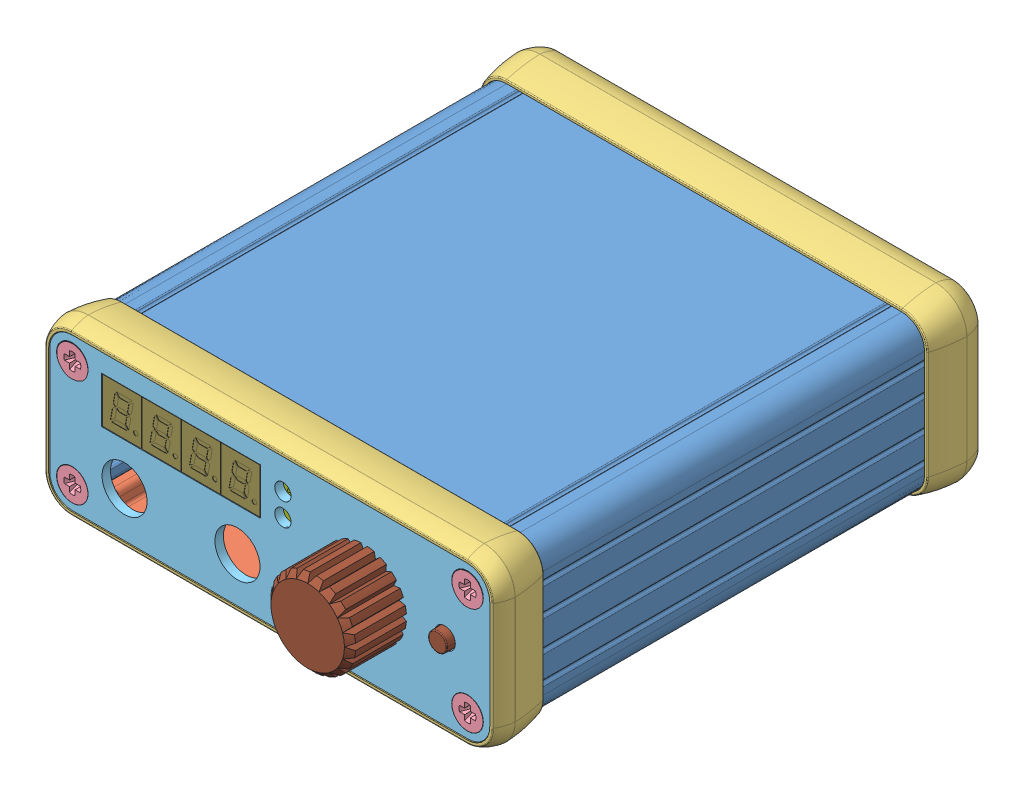
SolidWorks assembly Assembly_microbench_psu, configuration Standard. Lengths in mm. (continued)
Components (placement in the parent): (continued)
- main-board.step-1: main-board.step [Standard] at (-93.8915 -23.4474 -41.4) x (0 0 1) z (0 1 0) size (82.8 75 12.43) (continued)
  - R504.step-1: R504.step [Standard] at origin size (0.55 1.1 0.4) (continued)
    - 7876642432.step-1: 7876642432.step [Standard] at (25 39.4 0) x (0 1 0) z (0 0 1) size (1.1 0.55 0.4)
      - Terminal-12.step-1: Terminal-12.step [Standard] at (-0.55 -0.275 0) size (0.15 0.55 0.4)
        - Open CASCADE STEP translator 6.8 6.2.1-24.step-1: Open CASCADE STEP translator 6.8 6.2.1-24.step [Standard] at origin size (0.15 0.55 0.4)
      - Terminal-12.step-2: Terminal-12.step [Standard] at (0.55 0.275 0) x (-1 0 0) z (0 0 1) size (0.15 0.55 0.4)
        - Open CASCADE STEP translator 6.8 6.2.1-24.step-1: Open CASCADE STEP translator 6.8 6.2.1-24.step [Standard] at origin size (0.15 0.55 0.4)
      - Mid_Body-25.step-1: Mid_Body-25.step [Standard] at (-0.55 -0.275 0) size (1.02 0.55 0.32)
      - Mark-26.step-1: Mark-26.step [Standard] at (-0.4 -0.275 0.36) size (0.8 0.55 0.04)
  - R505.step-1: R505.step [Standard] at origin size (0.55 1.1 0.4)
    - 7876642992.step-1: 7876642992.step [Standard] at (15 43 0) x (0 -1 0) z (0 0 1) size (1.1 0.55 0.4)
      - Terminal-11.step-1: Terminal-11.step [Standard] at (-0.55 -0.275 0) size (0.15 0.55 0.4)
        - Open CASCADE STEP translator 6.8 6.2.1-21.step-1: Open CASCADE STEP translator 6.8 6.2.1-21.step [Standard] at origin size (0.15 0.55 0.4)
      - Terminal-11.step-2: Terminal-11.step [Standard] at (0.55 0.275 0) x (-1 0 0) z (0 0 1) size (0.15 0.55 0.4)
        - Open CASCADE STEP translator 6.8 6.2.1-21.step-1: Open CASCADE STEP translator 6.8 6.2.1-21.step [Standard] at origin size (0.15 0.55 0.4)
      - Mid_Body-22.step-1: Mid_Body-22.step [Standard] at (-0.55 -0.275 0) size (1.02 0.55 0.32)
      - Mark-23.step-1: Mark-23.step [Standard] at (-0.4 -0.275 0.36) size (0.8 0.55 0.04)
  - R506.step-1: R506.step [Standard] at origin size (1.1 0.55 0.4)
    - 7876648592.step-1: 7876648592.step [Standard] at (22 41.8 0) x (-1 0 0) z (0 0 1) size (1.1 0.55 0.4)
      - Terminal.step-1: Terminal.step [Standard] at (-0.55 -0.275 0) size (0.15 0.55 0.4)
        - Open CASCADE STEP translator 6.8 6.2.1.step-1: Open CASCADE STEP translator 6.8 6.2.1.step [Standard] at origin size (0.15 0.55 0.4)
      - Terminal.step-2: Terminal.step [Standard] at (0.55 0.275 0) x (-1 0 0) z (0 0 1) size (0.15 0.55 0.4)
        - Open CASCADE STEP translator 6.8 6.2.1.step-1: Open CASCADE STEP translator 6.8 6.2.1.step [Standard] at origin size (0.15 0.55 0.4)
      - Mid_Body.step-1: Mid_Body.step [Standard] at (-0.55 -0.275 0) size (1.02 0.55 0.32)
      - Mark.step-1: Mark.step [Standard] at (-0.4 -0.275 0.36) size (0.8 0.55 0.04)
  - R507.step-1: R507.step [Standard] at origin size (0.55 1.1 0.4)
    - 7876642432.step-1: 7876642432.step [Standard] at (21.6 43.2 0) x (0 1 0) z (0 0 1) size (1.1 0.55 0.4)
      - Terminal-12.step-1: Terminal-12.step [Standard] at (-0.55 -0.275 0) size (0.15 0.55 0.4)
        - Open CASCADE STEP translator 6.8 6.2.1-24.step-1: Open CASCADE STEP translator 6.8 6.2.1-24.step [Standard] at origin size (0.15 0.55 0.4)
      - Terminal-12.step-2: Terminal-12.step [Standard] at (0.55 0.275 0) x (-1 0 0) z (0 0 1) size (0.15 0.55 0.4)
        - Open CASCADE STEP translator 6.8 6.2.1-24.step-1: Open CASCADE STEP translator 6.8 6.2.1-24.step [Standard] at origin size (0.15 0.55 0.4)
      - Mid_Body-25.step-1: Mid_Body-25.step [Standard] at (-0.55 -0.275 0) size (1.02 0.55 0.32)
      - Mark-26.step-1: Mark-26.step [Standard] at (-0.4 -0.275 0.36) size (0.8 0.55 0.04)
  - R508.step-1: R508.step [Standard] at origin size (0.55 1.1 0.4)
    - 7876642992.step-1: 7876642992.step [Standard] at (21.2 38.4 0) x (0 -1 0) z (0 0 1) size (1.1 0.55 0.4)
      - Terminal-11.step-1: Terminal-11.step [Standard] at (-0.55 -0.275 0) size (0.15 0.55 0.4)
        - Open CASCADE STEP translator 6.8 6.2.1-21.step-1: Open CASCADE STEP translator 6.8 6.2.1-21.step [Standard] at origin size (0.15 0.55 0.4)
      - Terminal-11.step-2: Terminal-11.step [Standard] at (0.55 0.275 0) x (-1 0 0) z (0 0 1) size (0.15 0.55 0.4)
        - Open CASCADE STEP translator 6.8 6.2.1-21.step-1: Open CASCADE STEP translator 6.8 6.2.1-21.step [Standard] at origin size (0.15 0.55 0.4)
      - Mid_Body-22.step-1: Mid_Body-22.step [Standard] at (-0.55 -0.275 0) size (1.02 0.55 0.32)
      - Mark-23.step-1: Mark-23.step [Standard] at (-0.4 -0.275 0.36) size (0.8 0.55 0.04)
  - R509.step-1: R509.step [Standard] at origin size (1.1 0.55 0.4)
    - 7876648592.step-1: 7876648592.step [Standard] at (22 40.8 0) x (-1 0 0) z (0 0 1) size (1.1 0.55 0.4)
      - Terminal.step-1: Terminal.step [Standard] at (-0.55 -0.275 0) size (0.15 0.55 0.4)
        - Open CASCADE STEP translator 6.8 6.2.1.step-1: Open CASCADE STEP translator 6.8 6.2.1.step [Standard] at origin size (0.15 0.55 0.4)
      - Terminal.step-2: Terminal.step [Standard] at (0.55 0.275 0) x (-1 0 0) z (0 0 1) size (0.15 0.55 0.4)
        - Open CASCADE STEP translator 6.8 6.2.1.step-1: Open CASCADE STEP translator 6.8 6.2.1.step [Standard] at origin size (0.15 0.55 0.4)
      - Mid_Body.step-1: Mid_Body.step [Standard] at (-0.55 -0.275 0) size (1.02 0.55 0.32)
      - Mark.step-1: Mark.step [Standard] at (-0.4 -0.275 0.36) size (0.8 0.55 0.04)
  - R510.step-1: R510.step [Standard] at origin size (0.55 1.1 0.4)
    - 7876642432.step-1: 7876642432.step [Standard] at (20.2 36.6 0) x (0 1 0) z (0 0 1) size (1.1 0.55 0.4)
      - Terminal-12.step-1: Terminal-12.step [Standard] at (-0.55 -0.275 0) size (0.15 0.55 0.4)
        - Open CASCADE STEP translator 6.8 6.2.1-24.step-1: Open CASCADE STEP translator 6.8 6.2.1-24.step [Standard] at origin size (0.15 0.55 0.4)
      - Terminal-12.step-2: Terminal-12.step [Standard] at (0.55 0.275 0) x (-1 0 0) z (0 0 1) size (0.15 0.55 0.4)
        - Open CASCADE STEP translator 6.8 6.2.1-24.step-1: Open CASCADE STEP translator 6.8 6.2.1-24.step [Standard] at origin size (0.15 0.55 0.4)
      - Mid_Body-25.step-1: Mid_Body-25.step [Standard] at (-0.55 -0.275 0) size (1.02 0.55 0.32)
      - Mark-26.step-1: Mark-26.step [Standard] at (-0.4 -0.275 0.36) size (0.8 0.55 0.04)
  - R511.step-1: R511.step [Standard] at origin size (0.55 1.1 0.4)
    - 7876642992.step-1: 7876642992.step [Standard] at (19.2 43 0) x (0 -1 0) z (0 0 1) size (1.1 0.55 0.4)
      - Terminal-11.step-1: Terminal-11.step [Standard] at (-0.55 -0.275 0) size (0.15 0.55 0.4)
        - Open CASCADE STEP translator 6.8 6.2.1-21.step-1: Open CASCADE STEP translator 6.8 6.2.1-21.step [Standard] at origin size (0.15 0.55 0.4)
      - Terminal-11.step-2: Terminal-11.step [Standard] at (0.55 0.275 0) x (-1 0 0) z (0 0 1) size (0.15 0.55 0.4)
        - Open CASCADE STEP translator 6.8 6.2.1-21.step-1: Open CASCADE STEP translator 6.8 6.2.1-21.step [Standard] at origin size (0.15 0.55 0.4)
      - Mid_Body-22.step-1: Mid_Body-22.step [Standard] at (-0.55 -0.275 0) size (1.02 0.55 0.32)
      - Mark-23.step-1: Mark-23.step [Standard] at (-0.4 -0.275 0.36) size (0.8 0.55 0.04)
  - R512.step-1: R512.step [Standard] at origin size (1.1 0.55 0.4)
    - 7876648592.step-1: 7876648592.step [Standard] at (22 39.8 0) x (-1 0 0) z (0 0 1) size (1.1 0.55 0.4)
      - Terminal.step-1: Terminal.step [Standard] at (-0.55 -0.275 0) size (0.15 0.55 0.4)
        - Open CASCADE STEP translator 6.8 6.2.1.step-1: Open CASCADE STEP translator 6.8 6.2.1.step [Standard] at origin size (0.15 0.55 0.4)
      - Terminal.step-2: Terminal.step [Standard] at (0.55 0.275 0) x (-1 0 0) z (0 0 1) size (0.15 0.55 0.4)
        - Open CASCADE STEP translator 6.8 6.2.1.step-1: Open CASCADE STEP translator 6.8 6.2.1.step [Standard] at origin size (0.15 0.55 0.4)
      - Mid_Body.step-1: Mid_Body.step [Standard] at (-0.55 -0.275 0) size (1.02 0.55 0.32)
      - Mark.step-1: Mark.step [Standard] at (-0.4 -0.275 0.36) size (0.8 0.55 0.04)
  - TR500.step-1: TR500.step [Standard] at origin size (2.21 2.3 1.1)
    - 7556048800.step-1: 7556048800.step [Standard] at (23.1 37.5 0) x (0 -1 0) z (0 0 1) size (2.3 2.21 1.1)
      - Body.step-1: Body.step [Standard] at (-0.675 -1.1 0) size (1.35 2.21 1.1)
        - Open CASCADE STEP translator 7.5 3.1.1-27.step-1: Open CASCADE STEP translator 7.5 3.1.1-27.step [Standard] at origin size (1.35 2.21 1.1)
      - Leader.step-1: Leader.step [Standard] at (-0.675 -0.65 0) x (-1 0 0) z (0 0 1) size (0.47 0.4 0.6)
      - Leader.step-2: Leader.step [Standard] at (-0.675 0.65 0) x (-1 0 0) z (0 0 1) size (0.47 0.4 0.6)
      - Leader.step-3: Leader.step [Standard] at (0.675 0 0) size (0.47 0.4 0.6)
  - IC100.step-1: IC100.step [Standard] at origin size (4.39 4.39 0.9)
    - 7556051040.step-1: 7556051040.step [Standard] at (56.7 56.4 0) x (-0.707107 0.707107 0) z (0 0 1) size (3.1 3.1 0.9)
      - Body-1.step-1: Body-1.step [Standard] at (-1.55 -1.55 0) size (3.1 3.1 0.9)
        - Open CASCADE STEP translator 7.5 1.2.1-28.step-1: Open CASCADE STEP translator 7.5 1.2.1-28.step [Standard] at origin size (3.1 3.1 0.9)
      - Pin Shape.step-1: Pin Shape.step [Standard] at (-1.55 -0.9 0) size (0.4 0.2 0.2)
        - Open CASCADE STEP translator 7.5 1.4.1.step-1: Open CASCADE STEP translator 7.5 1.4.1.step [Standard] at origin size (0.4 0.2 0.2)
      - Pin Shape.step-2: Pin Shape.step [Standard] at (1.55 0.9 0) x (-1 0 0) z (0 0 1) size (0.4 0.2 0.2)
        - Open CASCADE STEP translator 7.5 1.4.1.step-1: Open CASCADE STEP translator 7.5 1.4.1.step [Standard] at origin size (0.4 0.2 0.2)
      - Pin Shape.step-3: Pin Shape.step [Standard] at (-1.55 -0.5 0) size (0.4 0.2 0.2)
        - Open CASCADE STEP translator 7.5 1.4.1.step-1: Open CASCADE STEP translator 7.5 1.4.1.step [Standard] at origin size (0.4 0.2 0.2)
      - Pin Shape.step-4: Pin Shape.step [Standard] at (1.55 0.5 0) x (-1 0 0) z (0 0 1) size (0.4 0.2 0.2)
        - Open CASCADE STEP translator 7.5 1.4.1.step-1: Open CASCADE STEP translator 7.5 1.4.1.step [Standard] at origin size (0.4 0.2 0.2)
      - Pin Shape.step-5: Pin Shape.step [Standard] at (-1.55 -0.1 0) size (0.4 0.2 0.2)
        - Open CASCADE STEP translator 7.5 1.4.1.step-1: Open CASCADE STEP translator 7.5 1.4.1.step [Standard] at origin size (0.4 0.2 0.2)
      - Pin Shape.step-6: Pin Shape.step [Standard] at (1.55 0.1 0) x (-1 0 0) z (0 0 1) size (0.4 0.2 0.2)
        - Open CASCADE STEP translator 7.5 1.4.1.step-1: Open CASCADE STEP translator 7.5 1.4.1.step [Standard] at origin size (0.4 0.2 0.2)
      - Pin Shape.step-7: Pin Shape.step [Standard] at (-1.55 0.3 0) size (0.4 0.2 0.2)
        - Open CASCADE STEP translator 7.5 1.4.1.step-1: Open CASCADE STEP translator 7.5 1.4.1.step [Standard] at origin size (0.4 0.2 0.2)
      - Pin Shape.step-8: Pin Shape.step [Standard] at (1.55 -0.3 0) x (-1 0 0) z (0 0 1) size (0.4 0.2 0.2)
        - Open CASCADE STEP translator 7.5 1.4.1.step-1: Open CASCADE STEP translator 7.5 1.4.1.step [Standard] at origin size (0.4 0.2 0.2)
      - Pin Shape.step-9: Pin Shape.step [Standard] at (-1.55 0.7 0) size (0.4 0.2 0.2)
        - Open CASCADE STEP translator 7.5 1.4.1.step-1: Open CASCADE STEP translator 7.5 1.4.1.step [Standard] at origin size (0.4 0.2 0.2)
      - Pin Shape.step-10: Pin Shape.step [Standard] at (1.55 -0.7 0) x (-1 0 0) z (0 0 1) size (0.4 0.2 0.2)
        - Open CASCADE STEP translator 7.5 1.4.1.step-1: Open CASCADE STEP translator 7.5 1.4.1.step [Standard] at origin size (0.4 0.2 0.2)
      - Pin Shape.step-11: Pin Shape.step [Standard] at (-0.7 -1.55 0) x (0 1 0) z (0 0 1) size (0.4 0.2 0.2)
        - Open CASCADE STEP translator 7.5 1.4.1.step-1: Open CASCADE STEP translator 7.5 1.4.1.step [Standard] at origin size (0.4 0.2 0.2)
      - Pin Shape.step-12: Pin Shape.step [Standard] at (0.7 1.55 0) x (0 -1 0) z (0 0 1) size (0.4 0.2 0.2)
        - Open CASCADE STEP translator 7.5 1.4.1.step-1: Open CASCADE STEP translator 7.5 1.4.1.step [Standard] at origin size (0.4 0.2 0.2)
      - Pin Shape.step-13: Pin Shape.step [Standard] at (-0.3 -1.55 0) x (0 1 0) z (0 0 1) size (0.4 0.2 0.2)
        - Open CASCADE STEP translator 7.5 1.4.1.step-1: Open CASCADE STEP translator 7.5 1.4.1.step [Standard] at origin size (0.4 0.2 0.2)
      - Pin Shape.step-14: Pin Shape.step [Standard] at (0.3 1.55 0) x (0 -1 0) z (0 0 1) size (0.4 0.2 0.2)
        - Open CASCADE STEP translator 7.5 1.4.1.step-1: Open CASCADE STEP translator 7.5 1.4.1.step [Standard] at origin size (0.4 0.2 0.2)
      - Pin Shape.step-15: Pin Shape.step [Standard] at (0.1 -1.55 0) x (0 1 0) z (0 0 1) size (0.4 0.2 0.2)
        - Open CASCADE STEP translator 7.5 1.4.1.step-1: Open CASCADE STEP translator 7.5 1.4.1.step [Standard] at origin size (0.4 0.2 0.2)
      - Pin Shape.step-16: Pin Shape.step [Standard] at (-0.1 1.55 0) x (0 -1 0) z (0 0 1) size (0.4 0.2 0.2)
        - Open CASCADE STEP translator 7.5 1.4.1.step-1: Open CASCADE STEP translator 7.5 1.4.1.step [Standard] at origin size (0.4 0.2 0.2)
      - Pin Shape.step-17: Pin Shape.step [Standard] at (0.5 -1.55 0) x (0 1 0) z (0 0 1) size (0.4 0.2 0.2)
        - Open CASCADE STEP translator 7.5 1.4.1.step-1: Open CASCADE STEP translator 7.5 1.4.1.step [Standard] at origin size (0.4 0.2 0.2)
      - Pin Shape.step-18: Pin Shape.step [Standard] at (-0.5 1.55 0) x (0 -1 0) z (0 0 1) size (0.4 0.2 0.2)
        - Open CASCADE STEP translator 7.5 1.4.1.step-1: Open CASCADE STEP translator 7.5 1.4.1.step [Standard] at origin size (0.4 0.2 0.2)
      - Pin Shape.step-19: Pin Shape.step [Standard] at (0.9 -1.55 0) x (0 1 0) z (0 0 1) size (0.4 0.2 0.2)
        - Open CASCADE STEP translator 7.5 1.4.1.step-1: Open CASCADE STEP translator 7.5 1.4.1.step [Standard] at origin size (0.4 0.2 0.2)
      - Pin Shape.step-20: Pin Shape.step [Standard] at (-0.9 1.55 0) x (0 -1 0) z (0 0 1) size (0.4 0.2 0.2)
        - Open CASCADE STEP translator 7.5 1.4.1.step-1: Open CASCADE STEP translator 7.5 1.4.1.step [Standard] at origin size (0.4 0.2 0.2)
      - Open CASCADE STEP translator 7.5 1.1.step-1: Open CASCADE STEP translator 7.5 1.1.step [Standard] at (-1.55 -1.55 0) size (0.4 0.4 0.01)
      - Thermal Shape.step-1: Thermal Shape.step [Standard] at (-0.85 -0.85 -0.001) size (1.7 1.7 0)
  - X104.step-1: X104.step [Standard] at origin size (5.5 3.81 4.5)
    - 20021121-00006XXLFc_RGB8421504.step-1: 20021121-00006XXLFc_RGB8421504.step [Standard] at (55.4 63.13 0.4127) x (0 1 0) z (1 0 0) size (3.81 4.5 5.5)
  - J100.step-1: J100.step [Standard] at origin size (14.7 12.4 12.2)
    - 54-00164_RGB8421504.step-1: 54-00164_RGB8421504.step [Standard] at (21.2172 3.7832 -4.8741) x (0 -1 0) z (-1 0 0) size (12.4 12.2 14.7)
      - 54-00164_shell.step-1: 54-00164_shell.step [Standard] at (-9.7167 10.3868 9.3173) size (9.6 12.2 12.5)
      - 54-00164_insulator.step-1: 54-00164_insulator.step [Standard] at (-9.7167 4.9868 9.3173) x (-1 0 0) z (0 0 -1) size (8.8 10.25 3.8)
      - 54-00164_center.step-1: 54-00164_center.step [Standard] at (-9.7167 11.3868 11.3173) x (-0.851288 0.524699 0) z (0 0 1) size (3.2 3.2 11.55)
      - 54-00164_center contact.step-1: 54-00164_center contact.step [Standard] at (-9.7167 11.3868 7.8173) x (-1 0 0) z (0 0 -1) size (8.6 8.9 9.55)
      - 54-00164_spring contact.step-1: 54-00164_spring contact.step [Standard] at (-9.7167 6.2868 13.6423) x (0 0 1) z (0 -1 0) size (10.74 9.62 4.55)
      - 54-00164_shell contact.step-1: 54-00164_shell contact.step [Standard] at (-9.0417 8.5868 10.3173) x (-1 0 0) z (0 1 0) size (9.75 2.7 4.05)
  - C306.step-1: C306.step [Standard] at origin size (8.3 9 10)
    - ChemiCon_HHXC500ARA470MHA0G_RGB8421504.step-1: ChemiCon_HHXC500ARA470MHA0G_RGB8421504.step [Standard] at (20.5 13.35 0) x (0 -1 0) z (0 0 1) size (9 8.3 10)
      - H-CHIP_D8_L10_ELEMENT.step-1: H-CHIP_D8_L10_ELEMENT.step [Standard] at origin size (8 8 9.35)
      - H-CHIP_D8_LEAD-.step-1: H-CHIP_D8_LEAD-.step [Standard] at origin size (2.96 0.91 2)
      - H-CHIP_D8_LEAD___.step-1: H-CHIP_D8_LEAD___.step [Standard] at origin size (2.96 0.91 2)
      - H-CHIP_D8_TABLE.step-1: H-CHIP_D8_TABLE.step [Standard] at origin size (8.3 8.3 2.31)
  - C303.step-1: C303.step [Standard] at origin size (8.3 9 10)
    - ChemiCon_HHXC500ARA470MHA0G_RGB8421504.step-1: ChemiCon_HHXC500ARA470MHA0G_RGB8421504.step [Standard] at (53.2 22.3 0) x (0 -1 0) z (0 0 1) size (9 8.3 10)
      - H-CHIP_D8_L10_ELEMENT.step-1: H-CHIP_D8_L10_ELEMENT.step [Standard] at origin size (8 8 9.35)
      - H-CHIP_D8_LEAD-.step-1: H-CHIP_D8_LEAD-.step [Standard] at origin size (2.96 0.91 2)
      - H-CHIP_D8_LEAD___.step-1: H-CHIP_D8_LEAD___.step [Standard] at origin size (2.96 0.91 2)
      - H-CHIP_D8_TABLE.step-1: H-CHIP_D8_TABLE.step [Standard] at origin size (8.3 8.3 2.31)
  - C302.step-1: C302.step [Standard] at origin size (8.3 9 10)
    - ChemiCon_HHXC500ARA470MHA0G_RGB8421504.step-1: ChemiCon_HHXC500ARA470MHA0G_RGB8421504.step [Standard] at (40.25 13 0) x (0 -1 0) z (0 0 1) size (9 8.3 10)
      - H-CHIP_D8_L10_ELEMENT.step-1: H-CHIP_D8_L10_ELEMENT.step [Standard] at origin size (8 8 9.35)
      - H-CHIP_D8_LEAD-.step-1: H-CHIP_D8_LEAD-.step [Standard] at origin size (2.96 0.91 2)
      - H-CHIP_D8_LEAD___.step-1: H-CHIP_D8_LEAD___.step [Standard] at origin size (2.96 0.91 2)
      - H-CHIP_D8_TABLE.step-1: H-CHIP_D8_TABLE.step [Standard] at origin size (8.3 8.3 2.31)
  - C100.step-1: C100.step [Standard] at origin size (1.27 1.27 0.65)
    - 7556052080.step-1: 7556052080.step [Standard] at (54.5 54.6 0) x (0.707107 -0.707107 0) z (0 0 1) size (1.15 0.65 0.65)
      - Terminal-13.step-1: Terminal-13.step [Standard] at (-0.575 -0.325 0) size (1.15 0.65 0.65)
        - Open CASCADE STEP translator 6.8 5.1.1-29.step-1: Open CASCADE STEP translator 6.8 5.1.1-29.step [Standard] at origin size (0.15 0.65 0.65)
        - Open CASCADE STEP translator 6.8 5.1.2-30.step-1: Open CASCADE STEP translator 6.8 5.1.2-30.step [Standard] at origin size (0.15 0.65 0.65)
      - Mid_Body-4.step-1: Mid_Body-4.step [Standard] at (-0.575 -0.325 0) size (0.85 0.65 0.65)
        - Open CASCADE STEP translator 6.8 5.2.1-31.step-1: Open CASCADE STEP translator 6.8 5.2.1-31.step [Standard] at origin size (0.85 0.65 0.65)
  - C403.step-1: C403.step [Standard] at origin size (0.65 1.15 0.65)
    - 7876639952.step-1: 7876639952.step [Standard] at (14.8 60.4 0) x (0 1 0) z (0 0 1) size (1.15 0.65 0.65)
      - Terminal-3.step-1: Terminal-3.step [Standard] at (-0.575 -0.325 0) size (1.15 0.65 0.65)
        - Open CASCADE STEP translator 6.8 5.1.1-4.step-1: Open CASCADE STEP translator 6.8 5.1.1-4.step [Standard] at origin size (0.15 0.65 0.65)
        - Open CASCADE STEP translator 6.8 5.1.2-5.step-1: Open CASCADE STEP translator 6.8 5.1.2-5.step [Standard] at origin size (0.15 0.65 0.65)
      - Mid_Body-2.step-1: Mid_Body-2.step [Standard] at (-0.575 -0.325 0) size (0.85 0.65 0.65)
        - Open CASCADE STEP translator 6.8 5.2.1-6.step-1: Open CASCADE STEP translator 6.8 5.2.1-6.step [Standard] at origin size (0.85 0.65 0.65)
  - C402.step-1: C402.step [Standard] at origin size (1.7 0.9 0.55)
    - 7556055920.step-1: 7556055920.step [Standard] at (12.8 60.2 0) x (-1 0 0) z (0 0 1) size (1.7 0.9 0.55)
      - Terminal-14.step-1: Terminal-14.step [Standard] at (-0.85 -0.45 0) size (0.1 0.9 0.55)
        - Open CASCADE STEP translator 7.5 6.2.1-32.step-1: Open CASCADE STEP translator 7.5 6.2.1-32.step [Standard] at origin size (0.1 0.9 0.55)
      - Terminal-14.step-2: Terminal-14.step [Standard] at (0.85 0.45 0) x (-1 0 0) z (0 0 1) size (0.1 0.9 0.55)
        - Open CASCADE STEP translator 7.5 6.2.1-32.step-1: Open CASCADE STEP translator 7.5 6.2.1-32.step [Standard] at origin size (0.1 0.9 0.55)
      - Mid Body-33.step-1: Mid Body-33.step [Standard] at (-0.85 -0.45 0) size (1.59 0.9 0.44)
      - Mark-34.step-1: Mark-34.step [Standard] at (-0.75 -0.45 0.495) size (1.5 0.9 0.06)
  - IC400.step-1: IC400.step [Standard] at origin size (3.1 2.1 1.05)
    - 7556047840.step-1: 7556047840.step [Standard] at (21 56.6 0) x (1 0 0) z (0 0 1) size (3.1 2.1 1.05)
      - Body-2.step-1: Body-2.step [Standard] at (-1.55 -1.05 0) size (3.1 2.1 1.05)
        - Open CASCADE STEP translator 7.5 3.2.1.step-1: Open CASCADE STEP translator 7.5 3.2.1.step [Standard] at origin size (3.1 2.1 1.05)
      - Pin Shape-1.step-1: Pin Shape-1.step [Standard] at (-1.55 -0.9 0) size (0.5 0.3 0.2)
        - Open CASCADE STEP translator 7.5 3.3.1.step-1: Open CASCADE STEP translator 7.5 3.3.1.step [Standard] at origin size (0.5 0.3 0.2)
      - Pin Shape-1.step-2: Pin Shape-1.step [Standard] at (-1.55 -0.4 0) size (0.5 0.3 0.2)
        - Open CASCADE STEP translator 7.5 3.3.1.step-1: Open CASCADE STEP translator 7.5 3.3.1.step [Standard] at origin size (0.5 0.3 0.2)
      - Pin Shape-1.step-3: Pin Shape-1.step [Standard] at (-1.55 0.1 0) size (0.5 0.3 0.2)
        - Open CASCADE STEP translator 7.5 3.3.1.step-1: Open CASCADE STEP translator 7.5 3.3.1.step [Standard] at origin size (0.5 0.3 0.2)
      - Pin Shape-1.step-4: Pin Shape-1.step [Standard] at (-1.55 0.6 0) size (0.5 0.3 0.2)
        - Open CASCADE STEP translator 7.5 3.3.1.step-1: Open CASCADE STEP translator 7.5 3.3.1.step [Standard] at origin size (0.5 0.3 0.2)
      - Pin Shape-1.step-5: Pin Shape-1.step [Standard] at (1.55 -0.6 0) x (-1 0 0) z (0 0 1) size (0.5 0.3 0.2)
        - Open CASCADE STEP translator 7.5 3.3.1.step-1: Open CASCADE STEP translator 7.5 3.3.1.step [Standard] at origin size (0.5 0.3 0.2)
      - Pin Shape-1.step-6: Pin Shape-1.step [Standard] at (1.55 -0.1 0) x (-1 0 0) z (0 0 1) size (0.5 0.3 0.2)
        - Open CASCADE STEP translator 7.5 3.3.1.step-1: Open CASCADE STEP translator 7.5 3.3.1.step [Standard] at origin size (0.5 0.3 0.2)
      - Pin Shape-1.step-7: Pin Shape-1.step [Standard] at (1.55 0.4 0) x (-1 0 0) z (0 0 1) size (0.5 0.3 0.2)
        - Open CASCADE STEP translator 7.5 3.3.1.step-1: Open CASCADE STEP translator 7.5 3.3.1.step [Standard] at origin size (0.5 0.3 0.2)
      - Pin Shape-1.step-8: Pin Shape-1.step [Standard] at (1.55 0.9 0) x (-1 0 0) z (0 0 1) size (0.5 0.3 0.2)
        - Open CASCADE STEP translator 7.5 3.3.1.step-1: Open CASCADE STEP translator 7.5 3.3.1.step [Standard] at origin size (0.5 0.3 0.2)
      - Open CASCADE STEP translator 7.5 3.1.step-1: Open CASCADE STEP translator 7.5 3.1.step [Standard] at (-1.55 -1.05 0) size (0.4 0.4 0.01)
  - C400.step-1: C400.step [Standard] at origin size (0.65 1.15 0.65)
    - 7876639952.step-1: 7876639952.step [Standard] at (19.6 58.8 0) x (0 1 0) z (0 0 1) size (1.15 0.65 0.65)
      - Terminal-3.step-1: Terminal-3.step [Standard] at (-0.575 -0.325 0) size (1.15 0.65 0.65)
        - Open CASCADE STEP translator 6.8 5.1.1-4.step-1: Open CASCADE STEP translator 6.8 5.1.1-4.step [Standard] at origin size (0.15 0.65 0.65)
        - Open CASCADE STEP translator 6.8 5.1.2-5.step-1: Open CASCADE STEP translator 6.8 5.1.2-5.step [Standard] at origin size (0.15 0.65 0.65)
      - Mid_Body-2.step-1: Mid_Body-2.step [Standard] at (-0.575 -0.325 0) size (0.85 0.65 0.65)
        - Open CASCADE STEP translator 6.8 5.2.1-6.step-1: Open CASCADE STEP translator 6.8 5.2.1-6.step [Standard] at origin size (0.85 0.65 0.65)
  - C401.step-1: C401.step [Standard] at origin size (1.15 0.65 0.65)
    - 7876636192.step-1: 7876636192.step [Standard] at (22.9 58.4 0) size (1.15 0.65 0.65)
      - Terminal-15.step-1: Terminal-15.step [Standard] at (-0.575 -0.325 0) size (1.15 0.65 0.65)
        - Open CASCADE STEP translator 6.8 5.1.1-35.step-1: Open CASCADE STEP translator 6.8 5.1.1-35.step [Standard] at origin size (0.15 0.65 0.65)
        - Open CASCADE STEP translator 6.8 5.1.2-36.step-1: Open CASCADE STEP translator 6.8 5.1.2-36.step [Standard] at origin size (0.15 0.65 0.65)
      - Mid_Body-5.step-1: Mid_Body-5.step [Standard] at (-0.575 -0.325 0) size (0.85 0.65 0.65)
        - Open CASCADE STEP translator 6.8 5.2.1-37.step-1: Open CASCADE STEP translator 6.8 5.2.1-37.step [Standard] at origin size (0.85 0.65 0.65)
  - X400.step-1: X400.step [Standard] at origin size (7.7 11.3 3.89)
    - USB4110-GF-A_RGB8421504.step-1: USB4110-GF-A_RGB8421504.step [Standard] at (0.15 56.9 0) x (0 -1 0) z (-1 0 0) size (11.3 3.89 7.7)
      - USB4110-GF-A_PART1.step-1: USB4110-GF-A_PART1.step [Standard] at (-4.47 -0.9 0) size (11.3 3.89 7.7)
  - R401.step-1: R401.step [Standard] at origin size (1.1 0.55 0.4)
    - 7876648592.step-1: 7876648592.step [Standard] at (5.7 49.6 0) x (-1 0 0) z (0 0 1) size (1.1 0.55 0.4)
      - Terminal.step-1: Terminal.step [Standard] at (-0.55 -0.275 0) size (0.15 0.55 0.4)
        - Open CASCADE STEP translator 6.8 6.2.1.step-1: Open CASCADE STEP translator 6.8 6.2.1.step [Standard] at origin size (0.15 0.55 0.4)
      - Terminal.step-2: Terminal.step [Standard] at (0.55 0.275 0) x (-1 0 0) z (0 0 1) size (0.15 0.55 0.4)
        - Open CASCADE STEP translator 6.8 6.2.1.step-1: Open CASCADE STEP translator 6.8 6.2.1.step [Standard] at origin size (0.15 0.55 0.4)
      - Mid_Body.step-1: Mid_Body.step [Standard] at (-0.55 -0.275 0) size (1.02 0.55 0.32)
      - Mark.step-1: Mark.step [Standard] at (-0.4 -0.275 0.36) size (0.8 0.55 0.04)
  - R400.step-1: R400.step [Standard] at origin size (1.1 0.55 0.4)
    - 7876648592.step-1: 7876648592.step [Standard] at (5.7 64.1 0) x (-1 0 0) z (0 0 1) size (1.1 0.55 0.4)
      - Terminal.step-1: Terminal.step [Standard] at (-0.55 -0.275 0) size (0.15 0.55 0.4)
        - Open CASCADE STEP translator 6.8 6.2.1.step-1: Open CASCADE STEP translator 6.8 6.2.1.step [Standard] at origin size (0.15 0.55 0.4)
      - Terminal.step-2: Terminal.step [Standard] at (0.55 0.275 0) x (-1 0 0) z (0 0 1) size (0.15 0.55 0.4)
        - Open CASCADE STEP translator 6.8 6.2.1.step-1: Open CASCADE STEP translator 6.8 6.2.1.step [Standard] at origin size (0.15 0.55 0.4)
      - Mid_Body.step-1: Mid_Body.step [Standard] at (-0.55 -0.275 0) size (1.02 0.55 0.32)
      - Mark.step-1: Mark.step [Standard] at (-0.4 -0.275 0.36) size (0.8 0.55 0.04)
  - IC401.step-1: IC401.step [Standard] at origin size (3 3 1)
    - 7556041840.step-1: 7556041840.step [Standard] at (12.8 57.4 0) x (0 -1 0) z (0 0 1) size (3 3 1)
      - Body-3.step-1: Body-3.step [Standard] at (-1.5 -1.5 0) size (3 3 1)
        - Open CASCADE STEP translator 7.5 1.2.1-38.step-1: Open CASCADE STEP translator 7.5 1.2.1-38.step [Standard] at origin size (3 3 1)
      - Open CASCADE STEP translator 7.5 1.1-39.step-1: Open CASCADE STEP translator 7.5 1.1-39.step [Standard] at (-1.5 -1.5 0) size (0.39 0.39 0.01)
      - Thermal Shape-40.step-1: Thermal Shape-40.step [Standard] at (-1.0375 -1.0375 -0.001) size (2.08 2.08 0)
  - TR303.step-1: TR303.step [Standard] at origin size (3.05 2.64 1.12)
    - 7556043920.step-1: 7556043920.step [Standard] at (49.5 32.8 0) x (0 -1 0) z (0 0 1) size (2.64 3.04 1.12)
      - Body-4.step-1: Body-4.step [Standard] at (-0.7 -1.52 0) size (1.41 3.04 1.11)
        - Open CASCADE STEP translator 7.5 1.1.1-41.step-1: Open CASCADE STEP translator 7.5 1.1.1-41.step [Standard] at origin size (1.41 3.04 1.11)
      - Leader-42.step-1: Leader-42.step [Standard] at (-0.7 -0.95 0) x (-1 0 0) z (0 0 1) size (0.62 0.5 0.61)
      - Leader-42.step-2: Leader-42.step [Standard] at (-0.7 0.95 0) x (-1 0 0) z (0 0 1) size (0.62 0.5 0.61)
      - Leader-42.step-3: Leader-42.step [Standard] at (0.7 0 0) size (0.62 0.5 0.61)
  - R307.step-1: R307.step [Standard] at origin size (0.55 1.1 0.4)
    - 7876642992.step-1: 7876642992.step [Standard] at (47.1 33.8 0) x (0 -1 0) z (0 0 1) size (1.1 0.55 0.4)
      - Terminal-11.step-1: Terminal-11.step [Standard] at (-0.55 -0.275 0) size (0.15 0.55 0.4)
        - Open CASCADE STEP translator 6.8 6.2.1-21.step-1: Open CASCADE STEP translator 6.8 6.2.1-21.step [Standard] at origin size (0.15 0.55 0.4)
      - Terminal-11.step-2: Terminal-11.step [Standard] at (0.55 0.275 0) x (-1 0 0) z (0 0 1) size (0.15 0.55 0.4)
        - Open CASCADE STEP translator 6.8 6.2.1-21.step-1: Open CASCADE STEP translator 6.8 6.2.1-21.step [Standard] at origin size (0.15 0.55 0.4)
      - Mid_Body-22.step-1: Mid_Body-22.step [Standard] at (-0.55 -0.275 0) size (1.02 0.55 0.32)
      - Mark-23.step-1: Mark-23.step [Standard] at (-0.4 -0.275 0.36) size (0.8 0.55 0.04)
  - R205.step-1: R205.step [Standard] at origin size (0.55 1.1 0.4)
    - 7876642992.step-1: 7876642992.step [Standard] at (31.1 52.9 0) x (0 -1 0) z (0 0 1) size (1.1 0.55 0.4)
      - Terminal-11.step-1: Terminal-11.step [Standard] at (-0.55 -0.275 0) size (0.15 0.55 0.4)
        - Open CASCADE STEP translator 6.8 6.2.1-21.step-1: Open CASCADE STEP translator 6.8 6.2.1-21.step [Standard] at origin size (0.15 0.55 0.4)
      - Terminal-11.step-2: Terminal-11.step [Standard] at (0.55 0.275 0) x (-1 0 0) z (0 0 1) size (0.15 0.55 0.4)
        - Open CASCADE STEP translator 6.8 6.2.1-21.step-1: Open CASCADE STEP translator 6.8 6.2.1-21.step [Standard] at origin size (0.15 0.55 0.4)
      - Mid_Body-22.step-1: Mid_Body-22.step [Standard] at (-0.55 -0.275 0) size (1.02 0.55 0.32)
      - Mark-23.step-1: Mark-23.step [Standard] at (-0.4 -0.275 0.36) size (0.8 0.55 0.04)
  - R204.step-1: R204.step [Standard] at origin size (0.55 1.1 0.4)
    - 7876642992.step-1: 7876642992.step [Standard] at (31.1 50.9 0) x (0 -1 0) z (0 0 1) size (1.1 0.55 0.4)
      - Terminal-11.step-1: Terminal-11.step [Standard] at (-0.55 -0.275 0) size (0.15 0.55 0.4)
        - Open CASCADE STEP translator 6.8 6.2.1-21.step-1: Open CASCADE STEP translator 6.8 6.2.1-21.step [Standard] at origin size (0.15 0.55 0.4)
      - Terminal-11.step-2: Terminal-11.step [Standard] at (0.55 0.275 0) x (-1 0 0) z (0 0 1) size (0.15 0.55 0.4)
        - Open CASCADE STEP translator 6.8 6.2.1-21.step-1: Open CASCADE STEP translator 6.8 6.2.1-21.step [Standard] at origin size (0.15 0.55 0.4)
      - Mid_Body-22.step-1: Mid_Body-22.step [Standard] at (-0.55 -0.275 0) size (1.02 0.55 0.32)
      - Mark-23.step-1: Mark-23.step [Standard] at (-0.4 -0.275 0.36) size (0.8 0.55 0.04)
  - R203.step-1: R203.step [Standard] at origin size (0.55 1.1 0.4)
    - 7876642992.step-1: 7876642992.step [Standard] at (31.2 64.5 0) x (0 -1 0) z (0 0 1) size (1.1 0.55 0.4)
      - Terminal-11.step-1: Terminal-11.step [Standard] at (-0.55 -0.275 0) size (0.15 0.55 0.4)
        - Open CASCADE STEP translator 6.8 6.2.1-21.step-1: Open CASCADE STEP translator 6.8 6.2.1-21.step [Standard] at origin size (0.15 0.55 0.4)
      - Terminal-11.step-2: Terminal-11.step [Standard] at (0.55 0.275 0) x (-1 0 0) z (0 0 1) size (0.15 0.55 0.4)
        - Open CASCADE STEP translator 6.8 6.2.1-21.step-1: Open CASCADE STEP translator 6.8 6.2.1-21.step [Standard] at origin size (0.15 0.55 0.4)
      - Mid_Body-22.step-1: Mid_Body-22.step [Standard] at (-0.55 -0.275 0) size (1.02 0.55 0.32)
      - Mark-23.step-1: Mark-23.step [Standard] at (-0.4 -0.275 0.36) size (0.8 0.55 0.04)
  - R202.step-1: R202.step [Standard] at origin size (0.55 1.1 0.4)
    - 7876642992.step-1: 7876642992.step [Standard] at (31.2 62.5 0) x (0 -1 0) z (0 0 1) size (1.1 0.55 0.4)
      - Terminal-11.step-1: Terminal-11.step [Standard] at (-0.55 -0.275 0) size (0.15 0.55 0.4)
        - Open CASCADE STEP translator 6.8 6.2.1-21.step-1: Open CASCADE STEP translator 6.8 6.2.1-21.step [Standard] at origin size (0.15 0.55 0.4)
      - Terminal-11.step-2: Terminal-11.step [Standard] at (0.55 0.275 0) x (-1 0 0) z (0 0 1) size (0.15 0.55 0.4)
        - Open CASCADE STEP translator 6.8 6.2.1-21.step-1: Open CASCADE STEP translator 6.8 6.2.1-21.step [Standard] at origin size (0.15 0.55 0.4)
      - Mid_Body-22.step-1: Mid_Body-22.step [Standard] at (-0.55 -0.275 0) size (1.02 0.55 0.32)
      - Mark-23.step-1: Mark-23.step [Standard] at (-0.4 -0.275 0.36) size (0.8 0.55 0.04)
  - R201.step-1: R201.step [Standard] at origin size (0.55 1.1 0.4)
    - 7876642992.step-1: 7876642992.step [Standard] at (43.146 64.533 0) x (0 -1 0) z (0 0 1) size (1.1 0.55 0.4)
      - Terminal-11.step-1: Terminal-11.step [Standard] at (-0.55 -0.275 0) size (0.15 0.55 0.4)
        - Open CASCADE STEP translator 6.8 6.2.1-21.step-1: Open CASCADE STEP translator 6.8 6.2.1-21.step [Standard] at origin size (0.15 0.55 0.4)
      - Terminal-11.step-2: Terminal-11.step [Standard] at (0.55 0.275 0) x (-1 0 0) z (0 0 1) size (0.15 0.55 0.4)
        - Open CASCADE STEP translator 6.8 6.2.1-21.step-1: Open CASCADE STEP translator 6.8 6.2.1-21.step [Standard] at origin size (0.15 0.55 0.4)
      - Mid_Body-22.step-1: Mid_Body-22.step [Standard] at (-0.55 -0.275 0) size (1.02 0.55 0.32)
      - Mark-23.step-1: Mark-23.step [Standard] at (-0.4 -0.275 0.36) size (0.8 0.55 0.04)
  - R200.step-1: R200.step [Standard] at origin size (0.55 1.1 0.4)
    - 7876642992.step-1: 7876642992.step [Standard] at (43.146 62.533 0) x (0 -1 0) z (0 0 1) size (1.1 0.55 0.4)
      - Terminal-11.step-1: Terminal-11.step [Standard] at (-0.55 -0.275 0) size (0.15 0.55 0.4)
        - Open CASCADE STEP translator 6.8 6.2.1-21.step-1: Open CASCADE STEP translator 6.8 6.2.1-21.step [Standard] at origin size (0.15 0.55 0.4)
      - Terminal-11.step-2: Terminal-11.step [Standard] at (0.55 0.275 0) x (-1 0 0) z (0 0 1) size (0.15 0.55 0.4)
        - Open CASCADE STEP translator 6.8 6.2.1-21.step-1: Open CASCADE STEP translator 6.8 6.2.1-21.step [Standard] at origin size (0.15 0.55 0.4)
      - Mid_Body-22.step-1: Mid_Body-22.step [Standard] at (-0.55 -0.275 0) size (1.02 0.55 0.32)
      - Mark-23.step-1: Mark-23.step [Standard] at (-0.4 -0.275 0.36) size (0.8 0.55 0.04)
  - L202.step-1: L202.step [Standard] at origin size (7.19 6.5 3.99)
    - SRP6540_RGB8421504.step-1: SRP6540_RGB8421504.step [Standard] at (29.5 46.3 2.2352) x (0 1 0) z (1 0 0) size (6.5 3.99 7.19)
  - L201.step-1: L201.step [Standard] at origin size (7.19 6.5 3.99)
    - SRP6540_RGB8421504.step-1: SRP6540_RGB8421504.step [Standard] at (29.4 57.9 2.2352) x (0 1 0) z (1 0 0) size (6.5 3.99 7.19)
  - L200.step-1: L200.step [Standard] at origin size (7.19 6.5 3.99)
    - SRP6540_RGB8421504.step-1: SRP6540_RGB8421504.step [Standard] at (41.3 57.9 2.2352) x (0 1 0) z (1 0 0) size (6.5 3.99 7.19)
  - IC202.step-1: IC202.step [Standard] at origin size (2.91 2.59 1.19)
    - 7556056800.step-1: 7556056800.step [Standard] at (27.7 51.9 0) x (0 -1 0) z (0 0 1) size (2.59 2.91 1.19)
      - Body-5.step-1: Body-5.step [Standard] at (-0.8 -1.45 0) size (1.6 2.91 1.13)
        - Open CASCADE STEP translator 7.5 7.1.1.step-1: Open CASCADE STEP translator 7.5 7.1.1.step [Standard] at origin size (1.6 2.91 1.13)
      - Leader-43.step-1: Leader-43.step [Standard] at (-0.8 -0.95 0) x (-1 0 0) z (0 0 1) size (0.6 0.46 0.68)
      - Leader-43.step-2: Leader-43.step [Standard] at (-0.8 0 0) x (-1 0 0) z (0 0 1) size (0.6 0.46 0.68)
      - Leader-43.step-3: Leader-43.step [Standard] at (-0.8 0.95 0) x (-1 0 0) z (0 0 1) size (0.6 0.46 0.68)
      - Leader-43.step-4: Leader-43.step [Standard] at (0.8 -0.95 0) size (0.6 0.46 0.68)
      - Leader-43.step-5: Leader-43.step [Standard] at (0.8 0 0) size (0.6 0.46 0.68)
      - Leader-43.step-6: Leader-43.step [Standard] at (0.8 0.95 0) size (0.6 0.46 0.68)
  - IC201.step-1: IC201.step [Standard] at origin size (2.91 2.59 1.19)
    - 7556056800.step-1: 7556056800.step [Standard] at (27.7 63.5 0) x (0 -1 0) z (0 0 1) size (2.59 2.91 1.19)
      - Body-5.step-1: Body-5.step [Standard] at (-0.8 -1.45 0) size (1.6 2.91 1.13)
        - Open CASCADE STEP translator 7.5 7.1.1.step-1: Open CASCADE STEP translator 7.5 7.1.1.step [Standard] at origin size (1.6 2.91 1.13)
      - Leader-43.step-1: Leader-43.step [Standard] at (-0.8 -0.95 0) x (-1 0 0) z (0 0 1) size (0.6 0.46 0.68)
      - Leader-43.step-2: Leader-43.step [Standard] at (-0.8 0 0) x (-1 0 0) z (0 0 1) size (0.6 0.46 0.68)
      - Leader-43.step-3: Leader-43.step [Standard] at (-0.8 0.95 0) x (-1 0 0) z (0 0 1) size (0.6 0.46 0.68)
      - Leader-43.step-4: Leader-43.step [Standard] at (0.8 -0.95 0) size (0.6 0.46 0.68)
      - Leader-43.step-5: Leader-43.step [Standard] at (0.8 0 0) size (0.6 0.46 0.68)
      - Leader-43.step-6: Leader-43.step [Standard] at (0.8 0.95 0) size (0.6 0.46 0.68)
  - IC200.step-1: IC200.step [Standard] at origin size (2.91 2.59 1.19)
    - 7556056800.step-1: 7556056800.step [Standard] at (39.746 63.533 0) x (0 -1 0) z (0 0 1) size (2.59 2.91 1.19)
      - Body-5.step-1: Body-5.step [Standard] at (-0.8 -1.45 0) size (1.6 2.91 1.13)
        - Open CASCADE STEP translator 7.5 7.1.1.step-1: Open CASCADE STEP translator 7.5 7.1.1.step [Standard] at origin size (1.6 2.91 1.13)
      - Leader-43.step-1: Leader-43.step [Standard] at (-0.8 -0.95 0) x (-1 0 0) z (0 0 1) size (0.6 0.46 0.68)
      - Leader-43.step-2: Leader-43.step [Standard] at (-0.8 0 0) x (-1 0 0) z (0 0 1) size (0.6 0.46 0.68)
      - Leader-43.step-3: Leader-43.step [Standard] at (-0.8 0.95 0) x (-1 0 0) z (0 0 1) size (0.6 0.46 0.68)
      - Leader-43.step-4: Leader-43.step [Standard] at (0.8 -0.95 0) size (0.6 0.46 0.68)
      - Leader-43.step-5: Leader-43.step [Standard] at (0.8 0 0) size (0.6 0.46 0.68)
      - Leader-43.step-6: Leader-43.step [Standard] at (0.8 0.95 0) size (0.6 0.46 0.68)
  - C301.step-1: C301.step [Standard] at origin size (0.65 1.15 0.65)
    - 7876647632.step-1: 7876647632.step [Standard] at (41.3 32.1 0) x (0 -1 0) z (0 0 1) size (1.15 0.65 0.65)
      - Terminal-6.step-1: Terminal-6.step [Standard] at (-0.575 -0.325 0) size (1.15 0.65 0.65)
        - Open CASCADE STEP translator 6.8 5.1.1-9.step-1: Open CASCADE STEP translator 6.8 5.1.1-9.step [Standard] at origin size (0.15 0.65 0.65)
        - Open CASCADE STEP translator 6.8 5.1.2-10.step-1: Open CASCADE STEP translator 6.8 5.1.2-10.step [Standard] at origin size (0.15 0.65 0.65)
      - Mid_Body-3.step-1: Mid_Body-3.step [Standard] at (-0.575 -0.325 0) size (0.85 0.65 0.65)
        - Open CASCADE STEP translator 6.8 5.2.1-11.step-1: Open CASCADE STEP translator 6.8 5.2.1-11.step [Standard] at origin size (0.85 0.65 0.65)
  - C211.step-1: C211.step [Standard] at origin size (1 1.8 1)
    - 7556047120.step-1: 7556047120.step [Standard] at (34.2 51.5 0) x (0 -1 0) z (0 0 1) size (1.8 1 1)
      - Terminal-16.step-1: Terminal-16.step [Standard] at (-0.9 -0.5 0) size (1.8 1 1)
        - Open CASCADE STEP translator 7.5 1.1.1-44.step-1: Open CASCADE STEP translator 7.5 1.1.1-44.step [Standard] at origin size (0.2 1 1)
        - Open CASCADE STEP translator 7.5 1.1.2-45.step-1: Open CASCADE STEP translator 7.5 1.1.2-45.step [Standard] at origin size (0.2 1 1)
      - Mid Body-3.step-1: Mid Body-3.step [Standard] at (-0.9 -0.5 0) size (1.4 1 1)
        - Open CASCADE STEP translator 7.5 1.2.1-46.step-1: Open CASCADE STEP translator 7.5 1.2.1-46.step [Standard] at origin size (1.4 1 1)
  - C210.step-1: C210.step [Standard] at origin size (1 1.8 1)
    - 7556047120.step-1: 7556047120.step [Standard] at (32.5 51.5 0) x (0 -1 0) z (0 0 1) size (1.8 1 1)
      - Terminal-16.step-1: Terminal-16.step [Standard] at (-0.9 -0.5 0) size (1.8 1 1)
        - Open CASCADE STEP translator 7.5 1.1.1-44.step-1: Open CASCADE STEP translator 7.5 1.1.1-44.step [Standard] at origin size (0.2 1 1)
        - Open CASCADE STEP translator 7.5 1.1.2-45.step-1: Open CASCADE STEP translator 7.5 1.1.2-45.step [Standard] at origin size (0.2 1 1)
      - Mid Body-3.step-1: Mid Body-3.step [Standard] at (-0.9 -0.5 0) size (1.4 1 1)
        - Open CASCADE STEP translator 7.5 1.2.1-46.step-1: Open CASCADE STEP translator 7.5 1.2.1-46.step [Standard] at origin size (1.4 1 1)
  - C209.step-1: C209.step [Standard] at origin size (0.65 1.15 0.65)
    - 7876639952.step-1: 7876639952.step [Standard] at (25.4 51.8 0) x (0 1 0) z (0 0 1) size (1.15 0.65 0.65)
      - Terminal-3.step-1: Terminal-3.step [Standard] at (-0.575 -0.325 0) size (1.15 0.65 0.65)
        - Open CASCADE STEP translator 6.8 5.1.1-4.step-1: Open CASCADE STEP translator 6.8 5.1.1-4.step [Standard] at origin size (0.15 0.65 0.65)
        - Open CASCADE STEP translator 6.8 5.1.2-5.step-1: Open CASCADE STEP translator 6.8 5.1.2-5.step [Standard] at origin size (0.15 0.65 0.65)
      - Mid_Body-2.step-1: Mid_Body-2.step [Standard] at (-0.575 -0.325 0) size (0.85 0.65 0.65)
        - Open CASCADE STEP translator 6.8 5.2.1-6.step-1: Open CASCADE STEP translator 6.8 5.2.1-6.step [Standard] at origin size (0.85 0.65 0.65)
  - C208.step-1: C208.step [Standard] at origin size (0.65 1.15 0.65)
    - 7876639952.step-1: 7876639952.step [Standard] at (30 50.9 0) x (0 1 0) z (0 0 1) size (1.15 0.65 0.65)
